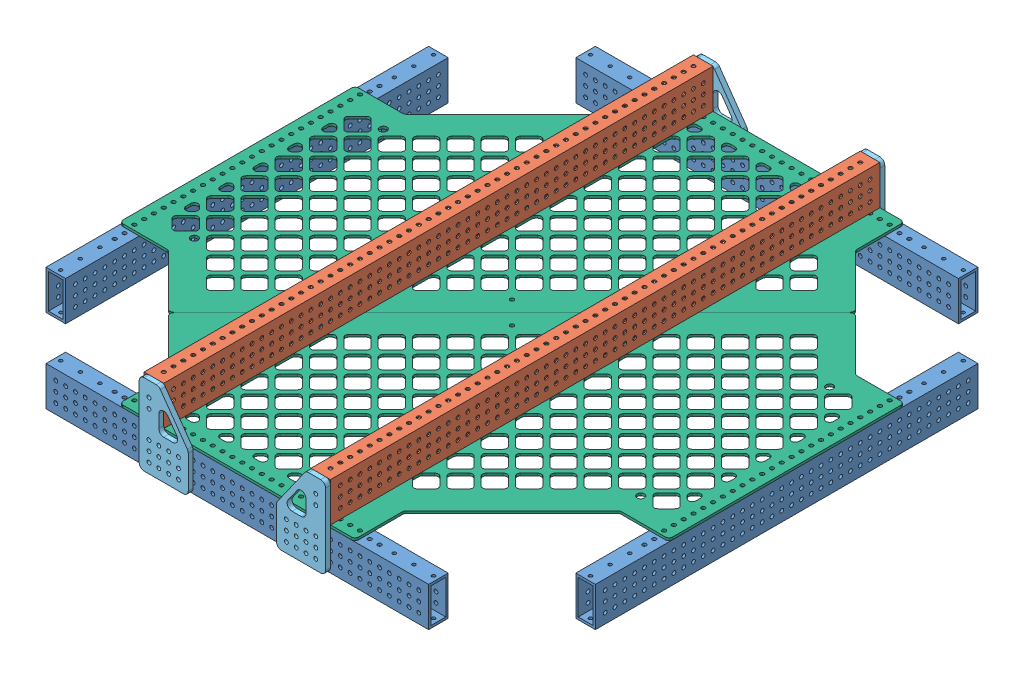
SolidWorks assembly 599-23-Prometheus-DT-A-0000, configuration Default. Lengths in mm.
Overall size (711.2 104.77 723.9).
20 component instances, 6 part files, 32 mates.
Components (placement in the parent):
- 599-23-Prometheus-DT-P-0001-1: 599-23-Prometheus-DT-P-0001 [Default] at (330.2 0 0) size (25.4 50.8 495.3)
- 599-23-Prometheus-DT-P-0001-2: 599-23-Prometheus-DT-P-0001 [Default] at (0 0 355.6) x (0 0 -1) z (1 0 0) size (25.4 50.8 495.3)
- 599-23-Prometheus-DT-P-0001-3: 599-23-Prometheus-DT-P-0001 [Default] at (-355.6 0 0) size (25.4 50.8 495.3)
- 599-23-Prometheus-DT-P-0001-4: 599-23-Prometheus-DT-P-0001 [Default] at (0 0 -355.6) x (0 0 1) z (-1 0 0) size (25.4 50.8 495.3)
- 599-23-Prometheus-DT-P-0002-1: 599-23-Prometheus-DT-P-0002 [Default] at (-120.65 53.975 0) size (25.4 50.8 711.2)
- 599-23-Prometheus-DT-P-0002-2: 599-23-Prometheus-DT-P-0002 [Default] at (95.25 53.975 0) size (25.4 50.8 711.2)
- 599-23-Prometheus-DT-P-0005-1: 599-23-Prometheus-DT-P-0005 [Default] at (-117.475 79.375 355.6) size (19.05 44.45 19.05)
- 599-23-Prometheus-DT-P-0008-1: 599-23-Prometheus-DT-P-0008 [Default] at (-119.0625 79.375 355.6) size (22.23 47.62 19.05)
- 599-23-Prometheus-DT-P-0006-1: 599-23-Prometheus-DT-P-0006 [Default] at (120.65 0 -358.775) x (-1 0 0) z (0 0 -1) size (63.5 104.77 6.35)
- 599-23-Prometheus-DT-P-0006-2: 599-23-Prometheus-DT-P-0006 [Default] at (-120.65 0 -358.775) size (63.5 104.77 6.35)
- 599-23-Prometheus-DT-P-0006-3: 599-23-Prometheus-DT-P-0006 [Default] at (120.65 0 358.775) x (-1 0 0) z (0 0 -1) size (63.5 104.77 6.35)
- 599-23-Prometheus-DT-P-0006-4: 599-23-Prometheus-DT-P-0006 [Default] at (-120.65 0 358.775) size (63.5 104.77 6.35)
- 599-23-Prometheus-DT-P-0003-1: 599-23-Prometheus-DT-P-0003 [Default] at (-355.6 50.8 355.6) size (575.62 3.17 575.62)
- 599-23-Prometheus-DT-P-0003-2: 599-23-Prometheus-DT-P-0003 [Default] at (355.6 50.8 -355.6) x (-1 0 0) z (0 0 -1) size (575.62 3.17 575.62)
- 599-23-Prometheus-DT-P-0005-5: 599-23-Prometheus-DT-P-0005 [Default] at (98.425 79.375 355.6) size (19.05 44.45 19.05)
- 599-23-Prometheus-DT-P-0008-2: 599-23-Prometheus-DT-P-0008 [Default] at (119.0625 79.375 336.55) x (-1 0 0) z (0 0 -1) size (22.23 47.62 19.05)
- 599-23-Prometheus-DT-P-0005-6: 599-23-Prometheus-DT-P-0005 [Default] at (-98.425 79.375 -355.6) x (-1 0 0) z (0 0 -1) size (19.05 44.45 19.05)
- 599-23-Prometheus-DT-P-0008-3: 599-23-Prometheus-DT-P-0008 [Default] at (-119.0625 79.375 -336.55) size (22.23 47.62 19.05)
- 599-23-Prometheus-DT-P-0005-7: 599-23-Prometheus-DT-P-0005 [Default] at (117.475 79.375 -355.6) x (-1 0 0) z (0 0 -1) size (19.05 44.45 19.05)
- 599-23-Prometheus-DT-P-0008-4: 599-23-Prometheus-DT-P-0008 [Default] at (119.0625 79.375 -355.6) x (-1 0 0) z (0 0 -1) size (22.23 47.62 19.05)
Mates (geometry in assembly coordinates):
- Coincident15: coincident anti-aligned: plane of 599-23-Prometheus-DT-P-0001-2 through (247.65 0 355.6) normal (0 -1 0)
- Symmetric1: symmetric aligned: plane of 599-23-Prometheus-DT-P-0001-2 through (247.65 0 355.6) normal (0 0 1); plane of 599-23-Prometheus-DT-P-0001-4 through (-247.65 0 -355.6) normal (0 0 -1)
- Symmetric2: symmetric aligned: plane of 599-23-Prometheus-DT-P-0001-1 through (355.6 0 247.65) normal (1 0 0); plane of 599-23-Prometheus-DT-P-0001-3 through (-355.6 0 247.65) normal (-1 0 0)
- Distance4: distance = 3.175 mm anti-aligned: plane of 599-23-Prometheus-DT-P-0001-4 through (-247.65 50.8 -355.6) normal (0 1 0); plane of 599-23-Prometheus-DT-P-0002-1 through (-120.65 53.975 355.6) normal (0 -1 0)
- Coincident17: coincident aligned: plane of 599-23-Prometheus-DT-P-0001-4 through (-247.65 0 -355.6) normal (0 0 -1); plane of 599-23-Prometheus-DT-P-0002-1 through (-120.65 53.975 -355.6) normal (0 0 -1)
- Distance3: distance = 3.175 mm anti-aligned: plane of 599-23-Prometheus-DT-P-0001-4 through (-247.65 50.8 -355.6) normal (0 1 0); plane of 599-23-Prometheus-DT-P-0002-2 through (95.25 53.975 355.6) normal (0 -1 0)
- Coincident19: coincident aligned: plane of 599-23-Prometheus-DT-P-0001-4 through (-247.65 0 -355.6) normal (0 0 -1); plane of 599-23-Prometheus-DT-P-0002-2 through (95.25 53.975 -355.6) normal (0 0 -1)
- Distance1: distance = 209.55 mm anti-aligned: plane of 599-23-Prometheus-DT-P-0001-3 through (-330.2 0 247.65) normal (1 0 0); plane of 599-23-Prometheus-DT-P-0002-1 through (-120.65 53.975 355.6) normal (-1 0 0)
- Distance2: distance = 209.55 mm anti-aligned: plane of 599-23-Prometheus-DT-P-0002-2 through (120.65 53.975 355.6) normal (1 0 0); plane of 599-23-Prometheus-DT-P-0001-1 through (330.2 0 247.65) normal (-1 0 0)
- Coincident20: coincident aligned: plane of 599-23-Prometheus-DT-P-0001-3 through (-355.6 0 247.65) normal (-1 0 0); plane of 599-23-Prometheus-DT-P-0003-1 through (-355.6 53.975 152.4) normal (-1 0 0)
- Coincident21: coincident anti-aligned: plane of 599-23-Prometheus-DT-P-0001-4 through (-247.65 50.8 -355.6) normal (0 1 0); plane of 599-23-Prometheus-DT-P-0003-1 through (-355.6 50.8 355.6) normal (0 -1 0)
- Coincident22: coincident aligned: plane of 599-23-Prometheus-DT-P-0001-4 through (-247.65 0 -355.6) normal (0 0 -1); plane of 599-23-Prometheus-DT-P-0003-1 through (-152.4 53.975 -355.6) normal (0 0 -1)
- Coincident26: coincident anti-aligned: plane of 599-23-Prometheus-DT-P-0001-2 through (247.65 50.8 355.6) normal (0 1 0); plane of 599-23-Prometheus-DT-P-0003-2 through (355.6 50.8 -355.6) normal (0 -1 0)
- Coincident27: coincident aligned: plane of 599-23-Prometheus-DT-P-0001-2 through (247.65 0 355.6) normal (0 0 1); plane of 599-23-Prometheus-DT-P-0003-2 through (152.4 53.975 355.6) normal (0 0 1)
- Coincident28: coincident aligned: plane of 599-23-Prometheus-DT-P-0001-1 through (355.6 0 247.65) normal (1 0 0); plane of 599-23-Prometheus-DT-P-0003-2 through (355.6 53.975 -152.4) normal (1 0 0)
- Coincident35: coincident aligned: plane of 599-23-Prometheus-DT-P-0002-1 through (-120.65 53.975 355.6) normal (0 0 1); plane of 599-23-Prometheus-DT-P-0005-1 through (-117.475 101.6 355.6) normal (0 0 1)
- Coincident36: coincident anti-aligned: plane of 599-23-Prometheus-DT-P-0008-1 through (-98.425 103.1875 355.6) normal (-1 0 0); plane of 599-23-Prometheus-DT-P-0005-1 through (-98.425 101.6 355.6) normal (1 0 0)
- Coincident37: coincident anti-aligned: plane of 599-23-Prometheus-DT-P-0008-1 through (-119.0625 101.6 355.6) normal (0 -1 0); plane of 599-23-Prometheus-DT-P-0005-1 through (-117.475 101.6 355.6) normal (0 1 0)
- Coincident47: coincident anti-aligned: plane of 599-23-Prometheus-DT-P-0006-1 through (120.65 0 -355.6) normal (0 0 1); plane of 599-23-Prometheus-DT-P-0001-4 through (-247.65 0 -355.6) normal (0 0 -1)
- Coincident48: coincident aligned: plane of 599-23-Prometheus-DT-P-0002-2 through (120.65 53.975 355.6) normal (1 0 0); plane of 599-23-Prometheus-DT-P-0006-1 through (120.65 0 -361.95) normal (1 0 0)
- Coincident49: coincident aligned: plane of 599-23-Prometheus-DT-P-0002-2 through (95.25 104.775 355.6) normal (0 1 0); plane of 599-23-Prometheus-DT-P-0006-1 through (120.65 104.775 -361.95) normal (0 1 0)
- Coincident50: coincident anti-aligned: plane of 599-23-Prometheus-DT-P-0001-4 through (-247.65 0 -355.6) normal (0 0 -1); plane of 599-23-Prometheus-DT-P-0006-2 through (-120.65 0 -355.6) normal (0 0 1)
- Coincident51: coincident aligned: plane of 599-23-Prometheus-DT-P-0002-1 through (-120.65 104.775 355.6) normal (0 1 0); plane of 599-23-Prometheus-DT-P-0006-2 through (-120.65 104.775 -355.6) normal (0 1 0)
- Coincident52: coincident aligned: plane of 599-23-Prometheus-DT-P-0002-1 through (-120.65 53.975 355.6) normal (-1 0 0); plane of 599-23-Prometheus-DT-P-0006-2 through (-120.65 0 -355.6) normal (-1 0 0)
- Coincident53: coincident aligned: plane of 599-23-Prometheus-DT-P-0002-2 through (95.25 104.775 355.6) normal (0 1 0); plane of 599-23-Prometheus-DT-P-0006-3 through (120.65 104.775 355.6) normal (0 1 0)
- Coincident55: coincident aligned: plane of 599-23-Prometheus-DT-P-0002-2 through (120.65 53.975 355.6) normal (1 0 0); plane of 599-23-Prometheus-DT-P-0006-3 through (120.65 0 355.6) normal (1 0 0)
- Coincident56: coincident aligned: plane of 599-23-Prometheus-DT-P-0002-1 through (-120.65 104.775 355.6) normal (0 1 0); plane of 599-23-Prometheus-DT-P-0006-4 through (-120.65 104.775 361.95) normal (0 1 0)
- Coincident57: coincident anti-aligned: plane of 599-23-Prometheus-DT-P-0002-1 through (-120.65 53.975 355.6) normal (0 0 1); plane of 599-23-Prometheus-DT-P-0006-4 through (-120.65 0 355.6) normal (0 0 -1)
- Coincident58: coincident aligned: plane of 599-23-Prometheus-DT-P-0002-1 through (-120.65 53.975 355.6) normal (-1 0 0); plane of 599-23-Prometheus-DT-P-0006-4 through (-120.65 0 361.95) normal (-1 0 0)
- Coincident81: coincident anti-aligned: plane of 599-23-Prometheus-DT-P-0002-1 through (-96.8375 55.5625 355.6) normal (-1 0 0); plane of 599-23-Prometheus-DT-P-0008-1 through (-96.8375 103.1875 355.6) normal (1 0 0)
- Coincident82: coincident aligned: plane of 599-23-Prometheus-DT-P-0005-1 through (-117.475 101.6 355.6) normal (0 0 1); plane of 599-23-Prometheus-DT-P-0008-1 through (-119.0625 103.1875 355.6) normal (0 0 1)
- Coincident83: coincident anti-aligned: plane of 599-23-Prometheus-DT-P-0002-1 through (-119.0625 55.5625 355.6) normal (0 1 0); plane of 599-23-Prometheus-DT-P-0008-1 through (-119.0625 55.5625 355.6) normal (0 -1 0)
